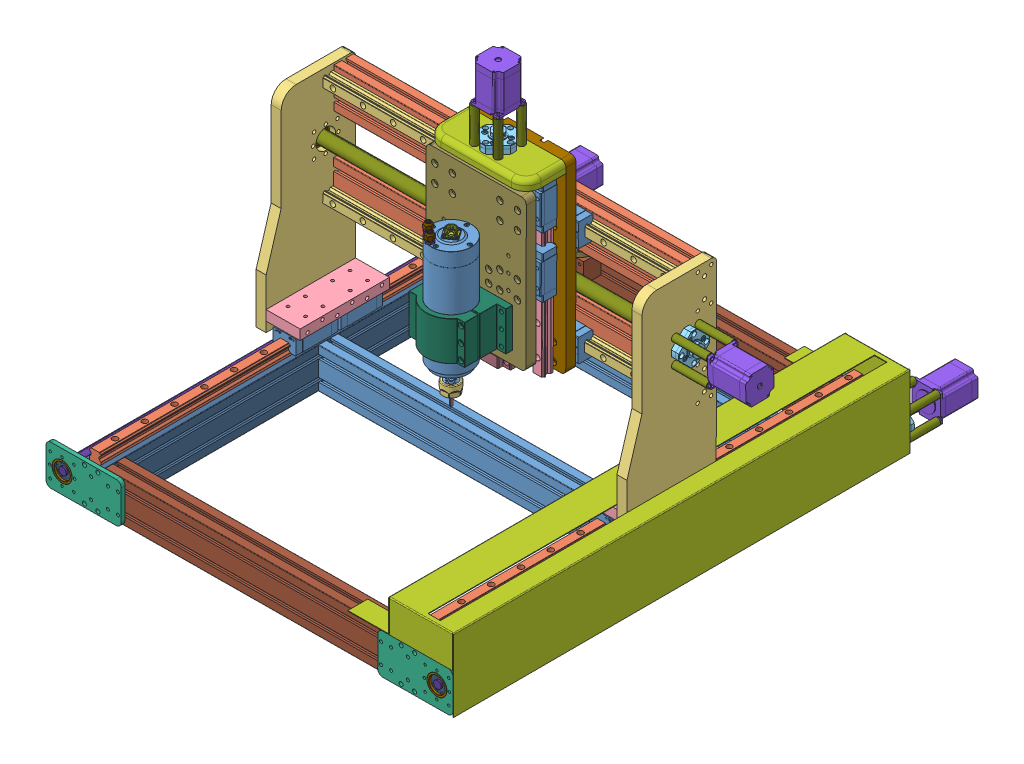
SolidWorks assembly cnc machine, configuration 默认. Lengths in mm.
Overall size (928.82 765.91 1084.64).
151 component instances, 43 part files, 170 mates.
Components (placement in the parent):
- HGH25CA-1: HGH25CA [Default] at (98.5712 571.5908 515.4933) x (0.999986 0.00209 -0.004953) z (0.004945 0.003582 0.999981) size (48 34.5 84.3)
- linerrailHGGR25-1: linerrailHGGR25 [默认] at (96.5872 570.1537 114.3088) x (0.999986 0.00209 -0.004953) z (0.004945 0.003582 0.999981) size (23 22 900)
- HGH25CA-2: HGH25CA [Default] at (98.1261 571.2684 425.495) x (0.999986 0.00209 -0.004953) z (0.004945 0.003582 0.999981) size (48 34.5 84.3)
- linerrailHGGR25-2: linerrailHGGR25 [默认] at (728.578 571.4746 111.1786) x (0.999986 0.00209 -0.004953) z (0.004945 0.003582 0.999981) size (23 22 900)
- HGH25CA-3: HGH25CA [Default] at (730.117 572.5893 422.3649) x (0.999986 0.00209 -0.004953) z (0.004945 0.003582 0.999981) size (48 34.5 84.3)
- HGH25CA-4: HGH25CA [Default] at (730.5621 572.9117 512.3632) x (0.999986 0.00209 -0.004953) z (0.004945 0.003582 0.999981) size (48 34.5 84.3)
- linerrailHGGR25400-2: linerrailHGGR25400 [默认] at (688.4331 946.5756 442.2318) x (0.002108 -0.999991 0.003572) z (-0.999986 -0.00209 0.004953) size (23 22 700)
- HGH25CA-5: HGH25CA [Default] at (543.984 946.2737 442.9472) x (0.002108 -0.999991 0.003572) z (-0.999986 -0.00209 0.004953) size (48 34.5 84.3)
- HGH25CA-6: HGH25CA [Default] at (427.9856 946.0312 443.5217) x (-0.002108 0.999991 -0.003572) z (0.999986 0.00209 -0.004953) size (48 34.5 84.3)
- HGH25CA-9: HGH25CA [Default] at (428.4072 746.033 444.236) x (-0.002108 0.999991 -0.003572) z (0.999986 0.00209 -0.004953) size (48 34.5 84.3)
- HGH25CA-10: HGH25CA [Default] at (544.4055 746.2754 443.6615) x (0.002108 -0.999991 0.003572) z (-0.999986 -0.00209 0.004953) size (48 34.5 84.3)
- linerrailHGGR25400-3: linerrailHGGR25400 [默认] at (688.8547 746.5773 442.9461) x (0.002108 -0.999991 0.003572) z (-0.999986 -0.00209 0.004953) size (23 22 700)
- linerrailHGGR25300-1: linerrailHGGR25300 [默认] at (421.1981 986.2312 503.4124) x (0.999986 0.00209 -0.004953) z (0.002108 -0.999991 0.003572) size (23 22 350)
- HGH25CA-11: HGH25CA [Default] at (421.3882 896.087 503.7344) x (0.999986 0.00209 -0.004953) z (0.002108 -0.999991 0.003572) size (48 34.5 84.3)
- HGH25CA-12: HGH25CA [Default] at (421.1352 1016.0859 503.3058) x (0.999986 0.00209 -0.004953) z (0.002108 -0.999991 0.003572) size (48 34.5 84.3)
- FK_15Yes_FS-1: FK_15Yes_FS [Default] at (783.6129 846.7535 436.1185) x (-0.004953 -0.000005 -0.999988) z (0.999986 0.00209 -0.004953) size (63 63 45.5)
  - _FK_15_FS_1_2-1: _FK_15_FS_1_2 [Default] x (0 0 -1) z (-1 0 0) size (41.5 63 63)
  - _FK_15collar_4-1: _FK_15collar_4 [Default] at (0 0 -11) x (0 0 -1) z (-1 0 0) size (10 19.5 19.5)
- top plate-1: top plate [默认] at (486.1176 1066.4308 520.8044) x (0.004945 0.003582 0.999981) z (-0.999986 -0.00209 0.004953) size (80 20 200)
- 57BYG250C-1: 57BYG250C [Default] at (485.8849 1167.4156 516.4438) x (-0.004945 -0.003582 -0.999981) z (-0.999986 -0.00209 0.004953) size (56.4 96.6 56.4)
- 57BYG250C-2: 57BYG250C [Default] at (37.9077 507.4456 -49.1795) x (-0.999986 -0.00209 0.004953) z (-0.002108 0.999991 -0.003572) size (56.4 96.6 56.4)
- 57BYG250C-3: 57BYG250C [Default] at (785.8969 509.0089 -52.8842) x (0.00471 -0.999983 0.003559) z (-0.999977 -0.004692 0.004962) size (56.4 96.6 56.4)
- FF_15-1: FF_15 [Default] at (42.7986 510.9881 939.8031) x (-0.004945 -0.003582 -0.999981) z (0.999959 -0.007604 -0.004918) size (17 63 63)
  - _FF_15Part1_2-1: _FF_15Part1_2 [Default] at origin size (17 63 63)
  - _FF_15_Part2_4-1: _FF_15_Part2_4 [Default] at (0.5 0 0) x (-1 0 0) z (0 0 1) size (9 32 32)
- sfu25unit-1: sfu25unit [默认] at (919.7497 -175.8868 131.6278) x (-0.999986 -0.00209 0.004953) z (-0.004945 -0.003582 -0.999981) size (51 66 50)
  - slidernutSLDPRT-1: slidernutSLDPRT [默认] at (903.5056 665.8309 -312.4749) x (0 1 0) z (0 0 1) size (66 48 40)
  - SFU2505-1: SFU2505 [默认] at (879.5056 685.8309 -262.4749) x (0 0 -1) z (1 0 0) size (42 60 51)
- FK_15Yes_FS-2: FK_15Yes_FS [Default] at (38.3082 507.7357 31.819) x (0.999986 0.00209 -0.004953) z (-0.004945 -0.003582 -0.999981) size (63 63 45.5)
  - _FK_15_FS_1_2-1: _FK_15_FS_1_2 [Default] x (0 0 -1) z (-1 0 0) size (41.5 63 63)
  - _FK_15collar_4-1: _FK_15collar_4 [Default] at (0 0 -11) x (0 0 -1) z (-1 0 0) size (10 19.5 19.5)
- 10mmwasher-1: 10mmwasher [默认] at (422.3231 1016.2241 541.3001) x (0.999986 0.00209 -0.004953) z (-0.002108 0.999991 -0.003572) size (50 20 58)
- sfu25unit-2: sfu25unit [默认] at (1223.1885 1158.8905 1278.7984) x (-0.004945 -0.003582 -0.999981) z (-0.008184 0.99996 -0.003541) size (51 66 50)
  - slidernutSLDPRT-1: slidernutSLDPRT [默认] at (903.5056 665.8309 -312.4749) x (0 1 0) z (0 0 1) size (66 48 40)
  - SFU2505-1: SFU2505 [默认] at (879.5056 685.8309 -262.4749) x (0 0 -1) z (1 0 0) size (42 60 51)
- nuts-1: nuts [默认] at (423.7205 738.6625 413.285) x (-0.002108 0.999991 -0.003572) z (0.999986 0.00209 -0.004953) size (14.5 9 300)
- nuts-2: nuts [默认] at (763.2635 953.8712 410.835) x (0.002108 -0.999991 0.003572) z (-0.999986 -0.00209 0.004953) size (14.5 9 300)
- 57BYG250C-4: 57BYG250C [Default] at (864.6117 846.9228 435.7173) x (-0.004979 0.012875 -0.999905) z (-0.002026 0.999915 0.012886) size (56.4 96.6 56.4)
- nuts-3: nuts [默认] at (739.2808 542.9437 796.2406) x (-0.999986 -0.00209 0.004953) z (-0.004945 -0.003582 -0.999981) size (14.5 9 300)
- nuts-4: nuts [默认] at (91.9989 541.0193 639.4456) x (0.999986 0.00209 -0.004953) z (0.004945 0.003582 0.999981) size (14.5 9 300)
- 80_2-1: 80_2 [По умолчанию] at (487.0688 826.6103 611.6604) x (-0.999986 -0.00209 0.004953) z (-0.002108 0.999991 -0.003572) size (147 100 78)
- FK_15Yes_FS-3: FK_15Yes_FS [Default] at (786.2974 509.2991 28.1143) x (0.999985 0.002163 -0.004953) z (-0.004945 -0.003582 -0.999981) size (63 63 45.5)
  - _FK_15_FS_1_2-1: _FK_15_FS_1_2 [Default] x (0 0 -1) z (-1 0 0) size (41.5 63 63)
  - _FK_15collar_4-1: _FK_15collar_4 [Default] at (0 0 -11) x (0 0 -1) z (-1 0 0) size (10 19.5 19.5)
- FF_15-2: FF_15 [Default] at (790.7877 512.5515 936.0974) x (-0.004945 -0.003582 -0.999981) z (0.99734 -0.072738 -0.004672) size (17 63 63)
  - _FF_15Part1_2-1: _FF_15Part1_2 [Default] at origin size (17 63 63)
  - _FF_15_Part2_4-1: _FF_15_Part2_4 [Default] at (0.5 0 0) x (-1 0 0) z (0 0 1) size (9 32 32)
- motor conectors-1: motor conectors [默认] at (551.7568 -126.7842 580.1434) x (0.997626 0.008459 -0.068346) z (0.066864 0.118667 0.99068) size (66.53 70.25 80.19)
  - motor connector-1: motor connector [默认] at (251.9755 716.8945 -454.5399) x (0.996395 -0.063381 0.056389) z (0.056389 0.991418 0.117947) size (14 70 14)
  - motor connector-2: motor connector [默认] at (251.6678 670.0654 -459.9605) x (0.996395 -0.063381 0.056389) z (0.056389 0.991418 0.117947) size (14 70 14)
  - motor connector-3: motor connector [默认] at (298.7148 669.4167 -457.0276) x (0.996395 -0.063381 0.056389) z (0.056389 0.991418 0.117947) size (14 70 14)
  - motor connector-4: motor connector [默认] at (299.0226 716.2459 -451.607) x (0.996395 -0.063381 0.056389) z (0.056389 0.991418 0.117947) size (14 70 14)
- motor conectors-2: motor conectors [默认] at (718.4868 1703.2016 -124.5715) x (-0.997788 -0.065443 0.011696) z (-0.063733 0.991691 0.111747) size (66.53 70.25 80.19)
  - motor connector-1: motor connector [默认] at (251.9755 716.8945 -454.5399) x (0.996395 -0.063381 0.056389) z (0.056389 0.991418 0.117947) size (14 70 14)
  - motor connector-2: motor connector [默认] at (251.6678 670.0654 -459.9605) x (0.996395 -0.063381 0.056389) z (0.056389 0.991418 0.117947) size (14 70 14)
  - motor connector-3: motor connector [默认] at (298.7148 669.4167 -457.0276) x (0.996395 -0.063381 0.056389) z (0.056389 0.991418 0.117947) size (14 70 14)
  - motor connector-4: motor connector [默认] at (299.0226 716.2459 -451.607) x (0.996395 -0.063381 0.056389) z (0.056389 0.991418 0.117947) size (14 70 14)
- motor conectors-3: motor conectors [默认] at (1404.6986 210.7802 671.758) x (-0.06833 0.003523 -0.997657) z (0.990854 0.116874 -0.067452) size (66.53 70.25 80.19)
  - motor connector-1: motor connector [默认] at (251.9755 716.8945 -454.5399) x (0.996395 -0.063381 0.056389) z (0.056389 0.991418 0.117947) size (14 70 14)
  - motor connector-2: motor connector [默认] at (251.6678 670.0654 -459.9605) x (0.996395 -0.063381 0.056389) z (0.056389 0.991418 0.117947) size (14 70 14)
  - motor connector-3: motor connector [默认] at (298.7148 669.4167 -457.0276) x (0.996395 -0.063381 0.056389) z (0.056389 0.991418 0.117947) size (14 70 14)
  - motor connector-4: motor connector [默认] at (299.0226 716.2459 -451.607) x (0.996395 -0.063381 0.056389) z (0.056389 0.991418 0.117947) size (14 70 14)
- FK_15Yes_FS-4: FK_15Yes_FS [Default] at (486.0557 1086.4163 516.7331) x (-0.004945 -0.003582 -0.999981) z (-0.002108 0.999991 -0.003572) size (63 63 45.5)
  - _FK_15_FS_1_2-1: _FK_15_FS_1_2 [Default] x (0 0 -1) z (-1 0 0) size (41.5 63 63)
  - _FK_15collar_4-1: _FK_15collar_4 [Default] at (0 0 -11) x (0 0 -1) z (-1 0 0) size (10 19.5 19.5)
- 80_2.2Kw-2: 80_2.2Kw [默认] at (40.2028 559.2798 2.5701) x (0.002108 -0.999991 0.003572) z (0.817895 -0.000331 -0.575368) size (312.58 80 86.72)
  - Шпиндель Ø80_2.2Kw.stp-1: Шпиндель Ø80_2.2Kw.stp [默认] at origin size (312.58 80 86.72)
    - Штуцер_1.stp-1: Штуцер_1.stp [默认] at (-415.6903 -776.6356 -7.6204) x (0 -0.235537 0.971865) z (-1 0 0) size (21.02 21.02 23.2)
      - штуцер.stp-1: штуцер.stp [默认] at (-4.5491 -1.5524 -3.4794) x (0.853763 -0.520662 0) z (0 0 1) size (13.95 16.11 23.2)
      - гайка штуцера.stp-1: гайка штуцера.stp [默认] at (-4.5491 -1.5524 10.3206) x (0.520662 0.853763 0) z (0 0 -1) size (13.95 16.11 11.51)
    - Штуцер_1.stp-2: Штуцер_1.stp [默认] at (-415.6903 -751.706 -14.3002) x (0 -0.235537 0.971865) z (-1 0 0) size (21.02 21.02 23.2)
      - штуцер.stp-1: штуцер.stp [默认] at (-4.5491 -1.5524 -3.4794) x (0.853763 -0.520662 0) z (0 0 1) size (13.95 16.11 23.2)
      - гайка штуцера.stp-1: гайка штуцера.stp [默认] at (-4.5491 -1.5524 10.3206) x (0.520662 0.853763 0) z (0 0 -1) size (13.95 16.11 11.51)
    - D880_2.2Kw.stp-1: D880_2.2Kw.stp [默认] at (-198.2109 -756.3828 14.95) x (-1 0 0) z (0 0 -1) size (258.95 80 80)
    - цанга ER20 6mm.stp-1: цанга ER20 6mm.stp [默认] at (-140.7359 -756.3828 14.95) x (-1 0 0) z (0 -0.095993 -0.995382) size (31.51 20.64 20.64)
    - Гайка ER20.stp-1: Гайка ER20.stp [默认] at (-163.2109 -756.3828 14.95) x (-1 0 0) z (0 -0.866025 -0.5) size (22.6 33.95 33.97)
    - фреза-01-01.stp-1: фреза-01-01.stp [默认] at (-118.2359 -756.3828 14.95) x (-1 0 0) z (0 -0.935872 -0.35234) size (51.4 6 6.02)
    - DIN 912 - M4 x 0,7 x 10 x 8,25.stp-1: DIN 912 - M4 x 0,7 x 10 x 8,25.stp [默认] at (-194.1109 -736.9328 -4.5) x (-1 0 0) z (0 0.013848 0.999904) size (14 7 7)
    - DIN 912 - M4 x 0,7 x 10 x 8,25.stp-2: DIN 912 - M4 x 0,7 x 10 x 8,25.stp [默认] at (-194.1109 -775.8328 -4.5) x (-1 0 0) z (0 0.006057 0.999982) size (14 7 7)
    - DIN 912 - M4 x 0,7 x 10 x 8,25.stp-3: DIN 912 - M4 x 0,7 x 10 x 8,25.stp [默认] at (-194.1109 -775.8328 34.4) x (-1 0 0) z (0 -0.004643 0.999989) size (14 7 7)
    - DIN 912 - M4 x 0,7 x 10 x 8,25.stp-4: DIN 912 - M4 x 0,7 x 10 x 8,25.stp [默认] at (-194.1109 -736.9328 34.4) x (-1 0 0) z (0 -0.003034 0.999995) size (14 7 7)
    - DIN 912 - M4 x 0,7 x 10 x 8,25.stp-5: DIN 912 - M4 x 0,7 x 10 x 8,25.stp [默认] at (-203.5909 -756.3828 -19.25) x (-1 0 0) z (0 -0.002194 0.999998) size (14 7 7)
    - DIN 912 - M4 x 0,7 x 10 x 8,25.stp-6: DIN 912 - M4 x 0,7 x 10 x 8,25.stp [默认] at (-203.5909 -790.5828 14.95) x (-1 0 0) z (0 -0.007324 0.999973) size (14 7 7)
    - DIN 912 - M4 x 0,7 x 10 x 8,25.stp-7: DIN 912 - M4 x 0,7 x 10 x 8,25.stp [默认] at (-203.5909 -722.1828 14.95) x (-1 0 0) z (0 0 1) size (14 7 7)
    - DIN 912 - M4 x 0,7 x 10 x 8,25.stp-8: DIN 912 - M4 x 0,7 x 10 x 8,25.stp [默认] at (-203.5909 -756.3828 49.15) x (-1 0 0) z (0 -0.007346 0.999973) size (14 7 7)
    - DIN 912 - M4 x 0,7 x 10 x 8,25.stp-9: DIN 912 - M4 x 0,7 x 10 x 8,25.stp [默认] at (-407.3109 -739.2828 -14.6681) size (14 7 7)
    - DIN 912 - M4 x 0,7 x 10 x 8,25.stp-10: DIN 912 - M4 x 0,7 x 10 x 8,25.stp [默认] at (-407.3109 -726.7648 32.05) size (14 7 7)
    - DIN 912 - M4 x 0,7 x 10 x 8,25.stp-11: DIN 912 - M4 x 0,7 x 10 x 8,25.stp [默认] at (-407.3109 -773.4828 44.5681) size (14 7 7)
    - DIN 912 - M4 x 0,7 x 10 x 8,25.stp-12: DIN 912 - M4 x 0,7 x 10 x 8,25.stp [默认] at (-407.3109 -786.0009 -2.15) size (14 7 7)
    - Прокладка разъема.stp-1: Прокладка разъема.stp [默认] at (-414.2109 -756.3828 14.95) x (0 0 1) z (-1 0 0) size (25.5 25.5 1.6)
    - штекер разъема.stp-1: штекер разъема.stp [默认] at (-415.8109 -756.3828 14.95) x (0 1 0) z (-1 0 0) size (24 24 21.5)
    - винт M3 x 12.stp-1: винт M3 x 12.stp [默认] at (-417.4109 -765.3828 5.95) size (14.38 5.6 5.6)
    - винт M3 x 12.stp-2: винт M3 x 12.stp [默认] at (-417.4109 -747.3828 5.95) size (14.38 5.6 5.6)
    - винт M3 x 12.stp-3: винт M3 x 12.stp [默认] at (-417.4109 -765.3828 23.95) size (14.38 5.6 5.6)
    - винт M3 x 12.stp-4: винт M3 x 12.stp [默认] at (-417.4109 -747.3828 23.95) size (14.38 5.6 5.6)
- back-2: back [默认] at (486.2676 901.289 481.3945) x (0.002108 -0.999991 0.003572) z (0.999986 0.00209 -0.004953) size (370 20 204.8)
- FF_15-3: FF_15 [Default] at (43.6235 845.2069 439.7836) x (-0.999986 -0.00209 0.004953) z (-0.002264 0.999373 -0.035332) size (17 63 63)
  - _FF_15Part1_2-1: _FF_15Part1_2 [Default] at origin size (17 63 63)
  - _FF_15_Part2_4-1: _FF_15_Part2_4 [Default] at (0.5 0 0) x (-1 0 0) z (0 0 1) size (9 32 32)
- bottom-1: bottom [默认] at (81.853 255.2246 4.6501) x (1 0.000018 0.000007) z (-0.000008 0.003582 0.999994) size (676.62 81.4 903.32)
  - EF4080-t5-900-1: EF4080-t5-900 [默认] at (14.5405 232.5342 35.786) x (-0.00209 0.999998 0.00001) z (0.004953 0 0.999988) size (80 40 900)
  - EF4080-t5-900-2: EF4080-t5-900 [默认] at (646.4477 273.8551 32.6562) x (0.00209 -0.999998 -0.00001) z (0.004953 0 0.999988) size (80 40 900)
  - EF4080-t5 -540-1: EF4080-t5 -540 [默认] at (630.8901 233.8133 912.7441) x (-0.00209 0.999998 0.00001) z (-0.999986 -0.00209 0.004953) size (80 40 592)
  - EF4080-t5 -540-2: EF4080-t5 -540 [默认] at (34.6392 232.576 55.6867) x (-0.00209 0.999998 0.00001) z (0.999986 0.00209 -0.004953) size (80 40 592)
- sfu25unit-3: sfu25unit [默认] at (-88.3542 -175.9045 721.574) x (0.999986 0.00209 -0.004953) z (0.004945 0.003582 0.999981) size (51 66 50)
  - slidernutSLDPRT-1: slidernutSLDPRT [默认] at (903.5056 665.8309 -312.4749) x (0 1 0) z (0 0 1) size (66 48 40)
  - SFU2505-1: SFU2505 [默认] at (879.5056 685.8309 -262.4749) x (0 0 -1) z (1 0 0) size (42 60 51)
- sfu25unit-4: sfu25unit [默认] at (784.4315 164.0685 1318.0819) x (-0.004945 -0.003582 -0.999981) z (0.999986 0.00209 -0.004953) size (51 66 50)
  - slidernutSLDPRT-1: slidernutSLDPRT [默认] at (903.5056 665.8309 -312.4749) x (0 1 0) z (0 0 1) size (66 48 40)
  - SFU2505-1: SFU2505 [默认] at (879.5056 685.8309 -262.4749) x (0 0 -1) z (1 0 0) size (42 60 51)
- sfu25unit-5: sfu25unit [默认] at (1176.0209 1188.3291 1392.4779) x (-0.004945 -0.003582 -0.999981) z (-0.002108 0.999991 -0.003572) size (51 66 50)
  - slidernutSLDPRT-1: slidernutSLDPRT [默认] at (903.5056 665.8309 -312.4749) x (0 1 0) z (0 0 1) size (66 48 40)
  - SFU2505-1: SFU2505 [默认] at (879.5056 685.8309 -262.4749) x (0 0 -1) z (1 0 0) size (42 60 51)
- motorseat-2: motorseat [默认] at (486.5435 911.3588 541.3582) x (-0.999986 -0.00209 0.004953) z (-0.002108 0.999991 -0.003572) size (200 20 300)
- linerrailHGGR25300-4: linerrailHGGR25300 [默认] at (551.1963 986.5029 502.7685) x (0.999986 0.00209 -0.004953) z (0.002108 -0.999991 0.003572) size (23 22 350)
- HGH25CA-16: HGH25CA [Default] at (551.3863 896.3587 503.0905) x (0.999986 0.00209 -0.004953) z (0.002108 -0.999991 0.003572) size (48 34.5 84.3)
- HGH25CA-17: HGH25CA [Default] at (551.1333 1016.3576 502.6619) x (0.999986 0.00209 -0.004953) z (0.002108 -0.999991 0.003572) size (48 34.5 84.3)
- motor conectors-4: motor conectors [默认] at (1123.8417 1707.1734 748.2712) x (-0.011299 -0.066969 -0.997691) z (-0.117376 0.990946 -0.065187) size (66.53 70.25 80.19)
  - motor connector-1: motor connector [默认] at (251.9755 716.8945 -454.5399) x (0.996395 -0.063381 0.056389) z (0.056389 0.991418 0.117947) size (14 70 14)
  - motor connector-2: motor connector [默认] at (251.6678 670.0654 -459.9605) x (0.996395 -0.063381 0.056389) z (0.056389 0.991418 0.117947) size (14 70 14)
  - motor connector-3: motor connector [默认] at (298.7148 669.4167 -457.0276) x (0.996395 -0.063381 0.056389) z (0.056389 0.991418 0.117947) size (14 70 14)
  - motor connector-4: motor connector [默认] at (299.0226 716.2459 -451.607) x (0.996395 -0.063381 0.056389) z (0.056389 0.991418 0.117947) size (14 70 14)
- BF_15-1: BF_15 [Default] at (486.8355 716.4195 518.0545) x (0.999986 0.00209 -0.004953) z (0.002108 -0.999991 0.003572) size (70 48 20)
  - _BF_15_Part1_2-1: _BF_15_Part1_2 [Default] at origin size (70 48 20)
  - _BF_15_Part2_4-1: _BF_15_Part2_4 [Default] at (0 0 -10) x (0 0 -1) z (-1 0 0) size (9 32 32)
- 8mmwasher-1: 8mmwasher [默认] at (486.6365 726.2338 482.0197) x (0.999988 -0.000009 -0.004945) z (0.000009 -0.999994 0.003582) size (70 8 20)
- screw2-1: screw2 [默认] at (34.6237 845.1881 439.8282) x (0.999986 0.00209 -0.004953) z (-0.004467 -0.189358 -0.981898) size (798 25 25)
- screw2 - right left-1: screw2 - right left [默认] at (790.8224 512.5765 943.0973) x (-0.004945 -0.003582 -0.999981) z (0.869601 0.493718 -0.006069) size (962 25 25)
- screw2 - right left-2: screw2 - right left [默认] at (42.8332 511.0132 946.8029) x (-0.004945 -0.003582 -0.999981) z (-0.951793 0.306719 0.003608) size (962 25 25)
- screw2 top-1: screw2 top [默认] at (486.8387 714.9195 518.0599) x (-0.002108 0.999991 -0.003572) z (0.052332 0.003677 0.998623) size (418 25 25)
- motor conectors-5: motor conectors [默认] at (-213.9124 -122.1999 583.9135) x (0.997448 -0.020988 -0.06824) z (0.070233 0.116788 0.99067) size (66.53 70.25 80.19)
  - motor connector-1: motor connector [默认] at (251.9755 716.8945 -454.5399) x (0.996395 -0.063381 0.056389) z (0.056389 0.991418 0.117947) size (14 70 14)
  - motor connector-2: motor connector [默认] at (251.6678 670.0654 -459.9605) x (0.996395 -0.063381 0.056389) z (0.056389 0.991418 0.117947) size (14 70 14)
  - motor connector-3: motor connector [默认] at (298.7148 669.4167 -457.0276) x (0.996395 -0.063381 0.056389) z (0.056389 0.991418 0.117947) size (14 70 14)
  - motor connector-4: motor connector [默认] at (299.0226 716.2459 -451.607) x (0.996395 -0.063381 0.056389) z (0.056389 0.991418 0.117947) size (14 70 14)
- EF4080-t5 -592-1: EF4080-t5 -592 [默认] at (117.0466 528.4647 189.4157) x (0.002108 -0.999991 0.003572) z (0.999986 0.00209 -0.004953) size (80 40 592)
- EF4080-t5 -592-2: EF4080-t5 -592 [默认] at (118.5302 529.5393 489.4101) x (0.002108 -0.999991 0.003572) z (0.999986 0.00209 -0.004953) size (80 40 592)
- EF4080-t5 -800-1: EF4080-t5 -800 [默认] at (63.3188 905.1192 403.4709) x (-0.002108 0.999991 -0.003572) z (0.999986 0.00209 -0.004953) size (80 40 700)
- EF4080-t5 -800-2: EF4080-t5 -800 [默认] at (63.656 745.1206 404.0424) x (-0.002108 0.999991 -0.003572) z (0.999986 0.00209 -0.004953) size (80 40 700)
- side right - final-5: side right - final [默认] at (43.7317 789.1036 437.9416) x (-0.004945 -0.003582 -0.999981) z (0.999986 0.00209 -0.004953) size (180 400 20)
- bottom-2: bottom [默认] at (98.3107 589.4294 470.4299) x (0.999986 0.00209 -0.004953) z (0.004945 0.003582 0.999981) size (68 20 180)
- conn12-1: conn12 [默认] at (73.866 589.0569 380.5504) x (0.004945 0.003582 0.999981) z (0.002108 -0.999991 0.003572) size (90 10 120)
- mot1-1: mot1 [默认] at (81.3076 507.8256 31.6061) x (-0.999986 -0.00209 0.004953) z (0.004945 0.003582 0.999981) size (150 80 8)
- side right - final-6: side right - final [默认] at (763.7213 790.6084 434.3756) x (-0.004945 -0.003582 -0.999981) z (0.999986 0.00209 -0.004953) size (180 400 20)
- bottom-3: bottom [默认] at (730.2594 610.7501 467.2283) x (0.999986 0.00209 -0.004953) z (-0.004945 -0.003582 -0.999981) size (68 20 180)
- conn12-2: conn12 [默认] at (754.3012 590.8005 467.1809) x (-0.004945 -0.003582 -0.999981) z (0.002108 -0.999991 0.003572) size (90 10 120)
- mot1-2: mot1 [默认] at (743.298 509.2092 28.3273) x (0.999986 0.00209 -0.004953) z (0.004945 0.003582 0.999981) size (150 80 8)
- mot1-3: mot1 [默认] at (747.7884 512.4616 936.3104) x (0.999986 0.00209 -0.004953) z (0.004945 0.003582 0.999981) size (150 80 8)
- mot1-4: mot1 [默认] at (85.7979 511.078 939.5891) x (-0.999986 -0.00209 0.004953) z (0.004945 0.003582 0.999981) size (150 80 8)
- track cover-1: track cover [默认] at (72.1405 614.9297 487.2762) x (-0.999986 -0.00209 0.004953) z (0.004945 0.003582 0.999981) size (210.94 145 920) (hidden)
- track cover-2: track cover [默认] at (756.5342 614.6651 483.8926) x (0.999986 0.00209 -0.004953) z (-0.004945 -0.003582 -0.999981) size (210.94 145 920)
Mates (geometry in assembly coordinates):
- Concentric1: concentric: cylinder of HGH25CA-1 through (86.9814 571.2054 486.5515) axis (0.004945 0.003582 0.999981) radius 2.43; cylinder of linerrailHGGR25-1 through (84.7699 569.6036 39.3668) axis (0.004945 0.003582 0.999981) radius 2.43
- Coincident17: coincident: plane of HGH25CA-1 through (90.0192 571.4693 486.5355) normal (0.002108 -0.999991 0.003572); plane of linerrailHGGR25-1 through (92.2585 573.0912 939.335) normal (-0.002108 0.999991 -0.003572)
- Concentric2: concentric: cylinder of linerrailHGGR25-1 through (107.6637 569.6515 39.2544) axis (0.004945 0.003582 0.999981) radius 2.43; cylinder of HGH25CA-2 through (109.4301 570.9309 396.4398) axis (0.004945 0.003582 0.999981) radius 2.43
- Coincident19: coincident: plane of linerrailHGGR25-1 through (92.2585 573.0912 939.335) normal (-0.002108 0.999991 -0.003572); plane of HGH25CA-2 through (89.5741 571.1469 396.5372) normal (0.002108 -0.999991 0.003572)
- Concentric3: concentric: cylinder of linerrailHGGR25-2 through (739.6546 570.9724 36.1242) axis (0.004945 0.003582 0.999981) radius 2.43; cylinder of HGH25CA-4 through (741.8661 572.5742 483.3079) axis (0.004945 0.003582 0.999981) radius 2.43
- Concentric4: concentric: cylinder of linerrailHGGR25-2 through (739.6546 570.9724 36.1242) axis (0.004945 0.003582 0.999981) radius 2.43; cylinder of HGH25CA-3 through (741.421 572.2518 393.3096) axis (0.004945 0.003582 0.999981) radius 2.43
- Coincident34: coincident: plane of linerrailHGGR25400-2 through (63.4244 953.6779 445.2972) normal (0.004945 0.003582 0.999981); plane of HGH25CA-6 through (399.0038 937.562 443.6954) normal (-0.004945 -0.003582 -0.999981)
- Concentric10: concentric: cylinder of linerrailHGGR25400-2 through (763.4076 958.1784 441.5619) axis (-0.999986 -0.00209 0.004953) radius 2.43; cylinder of HGH25CA-5 through (572.9581 957.7803 442.5052) axis (-0.999986 -0.00209 0.004953) radius 2.43
- Concentric12: concentric: cylinder of linerrailHGGR25300-1 through (432.4857 1061.2535 502.8303) axis (0.002108 -0.999991 0.003572) radius 2.43; cylinder of HGH25CA-11 through (432.7727 925.1097 503.3166) axis (0.002108 -0.999991 0.003572) radius 2.43
- Coincident41: coincident: plane of linerrailHGGR25300-1 through (413.3692 711.216 504.4362) normal (0.004945 0.003582 0.999981); plane of HGH25CA-11 through (412.9184 925.0691 503.6724) normal (-0.004945 -0.003582 -0.999981)
- Coincident92: coincident: plane of HGH25CA-9 through (399.4253 737.5637 444.4097) normal (-0.004945 -0.003582 -0.999981); plane of linerrailHGGR25400-3 through (63.846 753.6797 446.0115) normal (0.004945 0.003582 0.999981)
- Concentric14: concentric: cylinder of HGH25CA-10 through (573.3797 757.7821 443.2195) axis (-0.999986 -0.00209 0.004953) radius 2.43; cylinder of linerrailHGGR25400-3 through (763.8292 758.1801 442.2762) axis (-0.999986 -0.00209 0.004953) radius 2.43
- Concentric15: concentric: cylinder of HGH25CA-9 through (399.3822 757.4184 444.0813) axis (0.999986 0.00209 -0.004953) radius 2.43; cylinder of linerrailHGGR25400-3 through (763.8292 758.1801 442.2762) axis (-0.999986 -0.00209 0.004953) radius 2.43
- Concentric31: concentric: cylinder of linerrailHGGR25400-2 through (743.4323 946.6905 441.9594) axis (0.004945 0.003582 0.999981) radius 3.5; cylinder of nuts-2 through (741.84 945.5372 119.9654) axis (0.004945 0.003582 0.999981) radius 2.4112
- Concentric32: concentric: cylinder of linerrailHGGR25400-3 through (503.8573 746.1907 443.8623) axis (0.004945 0.003582 0.999981) radius 3.5; cylinder of nuts-1 through (502.265 745.0373 121.8683) axis (0.004945 0.003582 0.999981) radius 2.4112
- Concentric34: concentric: cylinder of FK_15Yes_FS-1/_FK_15_FS_1_2-1 through (800.6126 846.789 436.0343) axis (0.999986 0.00209 -0.004953) radius 6.9585; cylinder of 57BYG250C-4 through (833.0121 846.8568 435.8738) axis (0.999986 0.00209 -0.004953) radius 4
- Concentric35: concentric: cylinder of top plate-1 through (486.0978 1066.4165 516.8045) axis (-0.002108 0.999991 -0.003572) radius 20; cylinder of 57BYG250C-1 through (485.9515 1135.8159 516.5566) axis (-0.002108 0.999991 -0.003572) radius 4
- Concentric43: concentric: cylinder of 57BYG250C-2 through (38.0639 507.5588 -17.5801) axis (-0.004945 -0.003582 -0.999981) radius 4; cylinder of FK_15Yes_FS-2/_FK_15collar_4-1 through (38.4121 507.8109 52.8186) axis (-0.004945 -0.003582 -0.999981) radius 7.5
- Coincident242: coincident: plane of 57BYG250C-3 through (785.9513 509.0483 -41.8844) normal (0.004945 0.003582 0.999981); plane of motor conectors-1/motor connector-1 through (760.5735 532.9611 -41.8445) normal (-0.004945 -0.003582 -0.999981)
- Coincident243: coincident: plane of top plate-1 through (486.0755 1086.4307 520.733) normal (-0.002108 0.999991 -0.003572); plane of motor conectors-2/motor connector-2 through (509.5102 1086.3812 493.0453) normal (0.002108 -0.999991 0.003572)
- Concentric60: concentric: cylinder of top plate-1 through (462.6012 1086.4515 540.4208) axis (-0.002108 0.999991 -0.003572) radius 2.5; cylinder of motor conectors-2/motor connector-4 through (462.6012 1086.4515 540.4208) axis (-0.002108 0.999991 -0.003572) radius 7
- Concentric61: concentric: cylinder of top plate-1 through (509.7433 1086.55 540.1873) axis (-0.002108 0.999991 -0.003572) radius 2.5; cylinder of motor conectors-2/motor connector-1 through (509.7433 1086.55 540.1873) axis (-0.002108 0.999991 -0.003572) radius 7
- Parallel6: parallel: plane of top plate-1 through (386.2747 1086.3649 561.2275) normal (0.004945 0.003582 0.999981); plane of 57BYG250C-1 through (469.7129 1220.4823 544.5342) normal (0.004945 0.003582 0.999981)
- Coincident244: coincident: plane of 57BYG250C-1 through (485.9081 1156.4157 516.483) normal (0.002108 -0.999991 0.003572); plane of motor conectors-2/motor connector-4 through (462.4536 1156.4509 540.1708) normal (-0.002108 0.999991 -0.003572)
- Coincident246: coincident: plane of 57BYG250C-4 through (853.6118 846.8998 435.7718) normal (-0.999986 -0.00209 0.004953); plane of motor conectors-3/motor connector-4 through (853.4456 870.3852 412.1181) normal (0.999986 0.00209 -0.004953)
- Concentric74: concentric: cylinder of top plate-1 through (486.0978 1066.4165 516.8045) axis (-0.002108 0.999991 -0.003572) radius 20; cylinder of FK_15Yes_FS-4/_FK_15_FS_1_2-1 through (486.0915 1069.4165 516.7938) axis (-0.002108 0.999991 -0.003572) radius 20
- Coincident256: coincident: plane of top plate-1 through (486.0755 1086.4307 520.733) normal (-0.002108 0.999991 -0.003572); plane of FK_15Yes_FS-4/_FK_15_FS_1_2-1 through (517.0552 1086.4811 516.5795) normal (0.002108 -0.999991 0.003572)
- Concentric75: concentric: cylinder of top plate-1 through (486.1793 1086.5059 541.7326) axis (-0.002108 0.999991 -0.003572) radius 2.5; cylinder of FK_15Yes_FS-4/_FK_15_FS_1_2-1 through (486.1793 1086.5059 541.7326) axis (-0.002108 0.999991 -0.003572) radius 4.75
- Concentric85: concentric: cylinder of linerrailHGGR25400-2 through (683.4332 946.5651 442.2565) axis (0.004945 0.003582 0.999981) radius 3.5; cylinder of nuts-2 through (681.8408 945.4117 120.2625) axis (0.004945 0.003582 0.999981) radius 2.4112
- Concentric97: concentric: cylinder of 80_2-1 through (486.9866 865.6099 611.5211) axis (0.002108 -0.999991 0.003572) radius 40; cylinder of 80_2.2Kw-2/Шпиндель Ø80_2.2Kw.stp-1/D880_2.2Kw.stp-1 through (487.0118 853.66 611.5638) axis (-0.002108 0.999991 -0.003572) radius 40
- Coincident265: coincident: plane of linerrailHGGR25400-2 through (763.432 946.7323 441.8603) normal (0.999986 0.00209 -0.004953); plane of linerrailHGGR25400-3 through (763.8536 746.7341 442.5746) normal (0.999986 0.00209 -0.004953)
- Coincident267: coincident: plane of HGH25CA-5 through (573.0441 959.8987 460.755) normal (0.004945 0.003582 0.999981); plane of back-2 through (486.1687 901.2173 461.3948) normal (-0.004945 -0.003582 -0.999981)
- Concentric115: concentric: cylinder of HGH25CA-5 through (561.5358 963.8746 460.7977) axis (0.004945 0.003582 0.999981) radius 3; cylinder of back-2 through (561.6347 963.9462 480.7973) axis (0.004945 0.003582 0.999981) radius 6.5
- Concentric116: concentric: circle of HGH25CA-6; cylinder of back-2 through (410.6369 963.6306 481.5452) axis (0.004945 0.003582 0.999981) radius 3.3
- Coincident271: coincident: plane of top plate-1 through (385.8791 1086.0784 481.229) normal (-0.004945 -0.003582 -0.999981); plane of back-2 through (486.2676 901.289 481.3945) normal (0.004945 0.003582 0.999981)
- Coincident272: coincident: plane of linerrailHGGR25300-1 through (433.1688 711.1788 482.338) normal (-0.004945 -0.003582 -0.999981); plane of back-2 through (486.2676 901.289 481.3945) normal (0.004945 0.003582 0.999981)
- Concentric128: concentric: cylinder of linerrailHGGR25300-1 through (421.0822 1041.2307 503.216) axis (0.004945 0.003582 0.999981) radius 5.5; cylinder of back-2 through (420.8745 1041.0803 461.2168) axis (-0.004945 -0.003582 -0.999981) radius 2.5
- Coincident275: coincident: plane of top plate-1 through (586.2718 1086.7829 560.237) normal (0.999986 0.00209 -0.004953); plane of back-2 through (586.5572 716.4279 461.5603) normal (0.999986 0.00209 -0.004953)
- Coincident276: coincident: plane of top plate-1 through (486.0755 1086.4307 520.733) normal (-0.002108 0.999991 -0.003572); plane of back-2 through (585.7773 1086.4247 460.2388) normal (-0.002108 0.999991 -0.003572)
